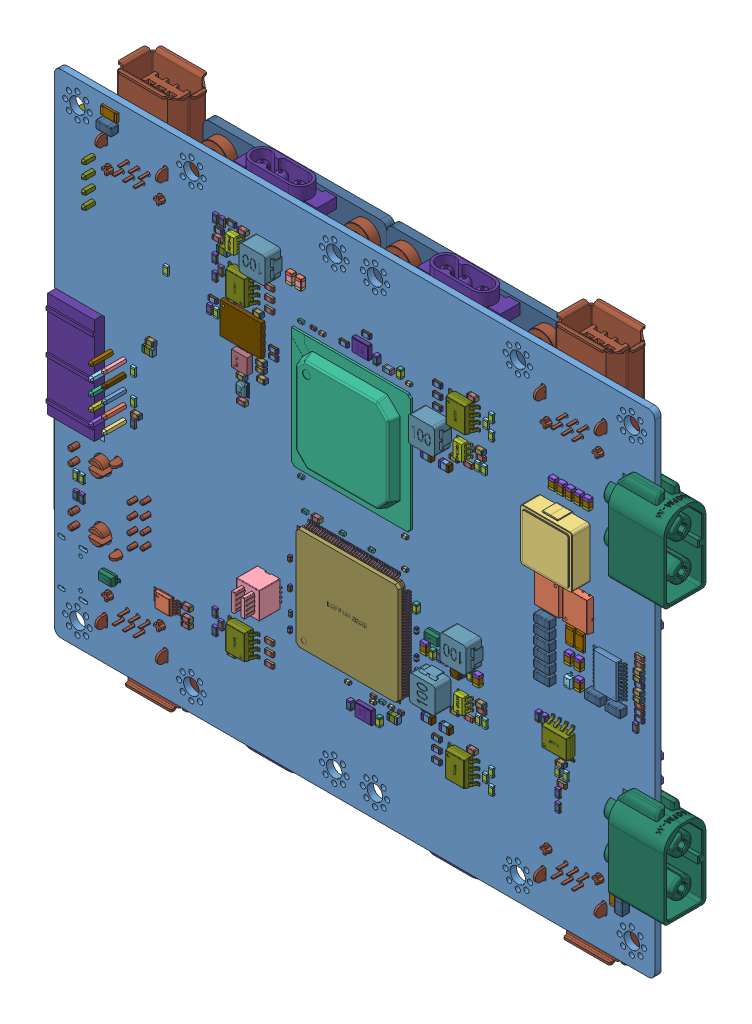
SolidWorks assembly Mother  Board, configuration 默认. Lengths in mm.
Overall size (122.6 102.08 21).
3917 component instances, 207 part files, 0 mates.
Components (placement in the parent):
- Mother  Board.step-1: Mother  Board.step [默认] at origin size (122.6 102.08 21)
  - Board.step-1: Board.step [默认] at origin size (115.82 95 1.22)
    - Open CASCADE STEP translator 6.8 1.1.1.step-1: Open CASCADE STEP translator 6.8 1.1.1.step [默认] at (0 0 -1.2164) size (115.82 95 1.22)
  - C149.step-1: C149.step [默认] at origin size (1.6 0.8 0.8)
    - 5993853984.step-1: 5993853984.step [默认] at (26.0351 21.4629 -1.2164) x (1 0 0) z (0 0 -1) size (1.6 0.8 0.8)
      - Terminal.step-1: Terminal.step [默认] at (-0.8 -0.4 0) size (1.6 0.8 0.8)
        - Open_CASCADE_STEP_translator_6.8_47.1.1.step-1: Open_CASCADE_STEP_translator_6.8_47.1.1.step [默认] at origin size (0.3 0.8 0.8)
        - Open_CASCADE_STEP_translator_6.8_47.1.2.step-1: Open_CASCADE_STEP_translator_6.8_47.1.2.step [默认] at origin size (0.3 0.8 0.8)
      - Mid_Body.step-1: Mid_Body.step [默认] at (-0.8 -0.4 0) size (1 0.8 0.8)
        - Open_CASCADE_STEP_translator_6.8_47.2.1.step-1: Open_CASCADE_STEP_translator_6.8_47.2.1.step [默认] at origin size (1 0.8 0.8)
  - R69.step-1: R69.step [默认] at origin size (1.6 0.8 0.45)
    - 5993853584.step-1: 5993853584.step [默认] at (108.2041 59.0549 -1.2164) x (1 0 0) z (0 0 -1) size (1.6 0.8 0.45)
      - Terminal-1.step-1: Terminal-1.step [默认] at (-0.8 -0.4 0) size (0.3 0.8 0.45)
        - Open_CASCADE_STEP_translator_6.8_21.2.1.step-1: Open_CASCADE_STEP_translator_6.8_21.2.1.step [默认] at origin size (0.3 0.8 0.45)
      - Terminal-1.step-2: Terminal-1.step [默认] at (0.8 0.4 0) x (-1 0 0) z (0 0 1) size (0.3 0.8 0.45)
        - Open_CASCADE_STEP_translator_6.8_21.2.1.step-1: Open_CASCADE_STEP_translator_6.8_21.2.1.step [默认] at origin size (0.3 0.8 0.45)
      - Mid_Body-0.step-1: Mid_Body-0.step [默认] at (-0.8 -0.4 0) size (1.51 0.8 0.36)
      - Mark.step-1: Mark.step [默认] at (-0.5 -0.4 0.405) size (1 0.8 0.05)
  - R68.step-1: R68.step [默认] at origin size (1.6 0.8 0.45)
    - 5993853584.step-1: 5993853584.step [默认] at (108.2041 54.9909 -1.2164) x (1 0 0) z (0 0 -1) size (1.6 0.8 0.45)
      - Terminal-1.step-1: Terminal-1.step [默认] at (-0.8 -0.4 0) size (0.3 0.8 0.45)
        - Open_CASCADE_STEP_translator_6.8_21.2.1.step-1: Open_CASCADE_STEP_translator_6.8_21.2.1.step [默认] at origin size (0.3 0.8 0.45)
      - Terminal-1.step-2: Terminal-1.step [默认] at (0.8 0.4 0) x (-1 0 0) z (0 0 1) size (0.3 0.8 0.45)
        - Open_CASCADE_STEP_translator_6.8_21.2.1.step-1: Open_CASCADE_STEP_translator_6.8_21.2.1.step [默认] at origin size (0.3 0.8 0.45)
      - Mid_Body-0.step-1: Mid_Body-0.step [默认] at (-0.8 -0.4 0) size (1.51 0.8 0.36)
      - Mark.step-1: Mark.step [默认] at (-0.5 -0.4 0.405) size (1 0.8 0.05)
  - R67.step-1: R67.step [默认] at origin size (1.6 0.8 0.45)
    - 5993853584.step-1: 5993853584.step [默认] at (108.2041 33.1469 -1.2164) x (1 0 0) z (0 0 -1) size (1.6 0.8 0.45)
      - Terminal-1.step-1: Terminal-1.step [默认] at (-0.8 -0.4 0) size (0.3 0.8 0.45)
        - Open_CASCADE_STEP_translator_6.8_21.2.1.step-1: Open_CASCADE_STEP_translator_6.8_21.2.1.step [默认] at origin size (0.3 0.8 0.45)
      - Terminal-1.step-2: Terminal-1.step [默认] at (0.8 0.4 0) x (-1 0 0) z (0 0 1) size (0.3 0.8 0.45)
        - Open_CASCADE_STEP_translator_6.8_21.2.1.step-1: Open_CASCADE_STEP_translator_6.8_21.2.1.step [默认] at origin size (0.3 0.8 0.45)
      - Mid_Body-0.step-1: Mid_Body-0.step [默认] at (-0.8 -0.4 0) size (1.51 0.8 0.36)
      - Mark.step-1: Mark.step [默认] at (-0.5 -0.4 0.405) size (1 0.8 0.05)
  - R66.step-1: R66.step [默认] at origin size (1.6 0.8 0.45)
    - 5993853584.step-1: 5993853584.step [默认] at (108.2041 28.9559 -1.2164) x (1 0 0) z (0 0 -1) size (1.6 0.8 0.45)
      - Terminal-1.step-1: Terminal-1.step [默认] at (-0.8 -0.4 0) size (0.3 0.8 0.45)
        - Open_CASCADE_STEP_translator_6.8_21.2.1.step-1: Open_CASCADE_STEP_translator_6.8_21.2.1.step [默认] at origin size (0.3 0.8 0.45)
      - Terminal-1.step-2: Terminal-1.step [默认] at (0.8 0.4 0) x (-1 0 0) z (0 0 1) size (0.3 0.8 0.45)
        - Open_CASCADE_STEP_translator_6.8_21.2.1.step-1: Open_CASCADE_STEP_translator_6.8_21.2.1.step [默认] at origin size (0.3 0.8 0.45)
      - Mid_Body-0.step-1: Mid_Body-0.step [默认] at (-0.8 -0.4 0) size (1.51 0.8 0.36)
      - Mark.step-1: Mark.step [默认] at (-0.5 -0.4 0.405) size (1 0.8 0.05)
  - LED4.step-1: LED4.step [默认] at origin size (1.16 1.62 0.6)
    - User_Library-GSideLED.step-1: User_Library-GSideLED.step [默认] at (109.6341 58.4995 -1.2164) x (0 1 0) z (0 0 -1) size (1.62 1.16 0.6)
  - LED3.step-1: LED3.step [默认] at origin size (1.16 1.62 0.6)
    - User_Library-GSideLED.step-1: User_Library-GSideLED.step [默认] at (109.6341 54.4355 -1.2164) x (0 1 0) z (0 0 -1) size (1.62 1.16 0.6)
  - LED2.step-1: LED2.step [默认] at origin size (1.16 1.62 0.6)
    - User_Library-GSideLED.step-1: User_Library-GSideLED.step [默认] at (109.6341 32.5915 -1.2164) x (0 1 0) z (0 0 -1) size (1.62 1.16 0.6)
  - LED1.step-1: LED1.step [默认] at origin size (1.16 1.62 0.6)
    - User_Library-GSideLED.step-1: User_Library-GSideLED.step [默认] at (109.6341 28.5275 -1.2164) x (0 1 0) z (0 0 -1) size (1.62 1.16 0.6)
  - R65.step-1: R65.step [默认] at origin size (3.1 1.55 0.47)
    - User_Library-R1206.step-1: User_Library-R1206.step [默认] at (6.4771 88.1381 0) x (1 0 0) z (0 0 1) size (3.1 1.55 0.47)
  - C148.step-1: C148.step [默认] at origin size (3 1.5 1.5)
    - (______).step-1: (______).step [默认] at (6.4769 86.2329 0) x (0 -1 0) z (0 0 1) size (1.5 3 1.5)
  - R64.step-1: R64.step [默认] at origin size (1.55 3.1 0.47)
    - User_Library-R1206.step-1: User_Library-R1206.step [默认] at (103.8859 5.9691 0) x (0 1 0) z (0 0 1) size (3.1 1.55 0.47)
  - C116.step-1: C116.step [默认] at origin size (1.5 3 1.5)
    - (______).step-1: (______).step [默认] at (105.7911 5.9689 0) x (1 0 0) z (0 0 1) size (1.5 3 1.5)
  - U10.step-1: U10.step [默认] at origin size (21.4 15.88 16.5)
    - HanRun-HR911105A.step-1: HanRun-HR911105A.step [默认] at (-6.0265 14.8679 -15) x (0 1 0) z (-1 0 0) size (15.88 16.5 21.4)
  - U15.step-1: U15.step [默认] at origin size (22 22 1.45)
    - LQFP144-20x20.step-1: LQFP144-20x20.step [默认] at (53.4654 28.321 0) x (1 0 0) z (0 0 1) size (22 22 1.45)
      - LQFP144_20x20______.step-1: LQFP144_20x20______.step [默认] at origin size (20 20 1.4)
      - _____0.25.step-1: _____0.25.step [默认] at (8.75 -11 0.05) x (-1 0 0) z (0 0 -1) size (0.25 1.2 0.8)
      - _____0.25.step-2: _____0.25.step [默认] at (8.25 -11 0.05) x (-1 0 0) z (0 0 -1) size (0.25 1.2 0.8)
      - _____0.25.step-3: _____0.25.step [默认] at (7.75 -11 0.05) x (-1 0 0) z (0 0 -1) size (0.25 1.2 0.8)
      - _____0.25.step-4: _____0.25.step [默认] at (7.25 -11 0.05) x (-1 0 0) z (0 0 -1) size (0.25 1.2 0.8)
      - _____0.25.step-5: _____0.25.step [默认] at (6.75 -11 0.05) x (-1 0 0) z (0 0 -1) size (0.25 1.2 0.8)
      - _____0.25.step-6: _____0.25.step [默认] at (6.25 -11 0.05) x (-1 0 0) z (0 0 -1) size (0.25 1.2 0.8)
      - _____0.25.step-7: _____0.25.step [默认] at (5.75 -11 0.05) x (-1 0 0) z (0 0 -1) size (0.25 1.2 0.8)
      - _____0.25.step-8: _____0.25.step [默认] at (5.25 -11 0.05) x (-1 0 0) z (0 0 -1) size (0.25 1.2 0.8)
      - _____0.25.step-9: _____0.25.step [默认] at (4.75 -11 0.05) x (-1 0 0) z (0 0 -1) size (0.25 1.2 0.8)
      - _____0.25.step-10: _____0.25.step [默认] at (4.25 -11 0.05) x (-1 0 0) z (0 0 -1) size (0.25 1.2 0.8)
      - _____0.25.step-11: _____0.25.step [默认] at (3.75 -11 0.05) x (-1 0 0) z (0 0 -1) size (0.25 1.2 0.8)
      - _____0.25.step-12: _____0.25.step [默认] at (3.25 -11 0.05) x (-1 0 0) z (0 0 -1) size (0.25 1.2 0.8)
      - _____0.25.step-13: _____0.25.step [默认] at (2.75 -11 0.05) x (-1 0 0) z (0 0 -1) size (0.25 1.2 0.8)
      - _____0.25.step-14: _____0.25.step [默认] at (2.25 -11 0.05) x (-1 0 0) z (0 0 -1) size (0.25 1.2 0.8)
      - _____0.25.step-15: _____0.25.step [默认] at (1.75 -11 0.05) x (-1 0 0) z (0 0 -1) size (0.25 1.2 0.8)
      - _____0.25.step-16: _____0.25.step [默认] at (1.25 -11 0.05) x (-1 0 0) z (0 0 -1) size (0.25 1.2 0.8)
      - _____0.25.step-17: _____0.25.step [默认] at (0.75 -11 0.05) x (-1 0 0) z (0 0 -1) size (0.25 1.2 0.8)
      - _____0.25.step-18: _____0.25.step [默认] at (0.25 -11 0.05) x (-1 0 0) z (0 0 -1) size (0.25 1.2 0.8)
      - _____0.25.step-19: _____0.25.step [默认] at (-0.25 -11 0.05) x (-1 0 0) z (0 0 -1) size (0.25 1.2 0.8)
      - _____0.25.step-20: _____0.25.step [默认] at (-0.75 -11 0.05) x (-1 0 0) z (0 0 -1) size (0.25 1.2 0.8)
      - _____0.25.step-21: _____0.25.step [默认] at (-1.25 -11 0.05) x (-1 0 0) z (0 0 -1) size (0.25 1.2 0.8)
      - _____0.25.step-22: _____0.25.step [默认] at (-1.75 -11 0.05) x (-1 0 0) z (0 0 -1) size (0.25 1.2 0.8)
      - _____0.25.step-23: _____0.25.step [默认] at (-2.25 -11 0.05) x (-1 0 0) z (0 0 -1) size (0.25 1.2 0.8)
      - _____0.25.step-24: _____0.25.step [默认] at (-2.75 -11 0.05) x (-1 0 0) z (0 0 -1) size (0.25 1.2 0.8)
      - _____0.25.step-25: _____0.25.step [默认] at (-3.25 -11 0.05) x (-1 0 0) z (0 0 -1) size (0.25 1.2 0.8)
      - _____0.25.step-26: _____0.25.step [默认] at (-3.75 -11 0.05) x (-1 0 0) z (0 0 -1) size (0.25 1.2 0.8)
      - _____0.25.step-27: _____0.25.step [默认] at (-4.25 -11 0.05) x (-1 0 0) z (0 0 -1) size (0.25 1.2 0.8)
      - _____0.25.step-28: _____0.25.step [默认] at (-4.75 -11 0.05) x (-1 0 0) z (0 0 -1) size (0.25 1.2 0.8)
      - _____0.25.step-29: _____0.25.step [默认] at (-5.25 -11 0.05) x (-1 0 0) z (0 0 -1) size (0.25 1.2 0.8)
      - _____0.25.step-30: _____0.25.step [默认] at (-5.75 -11 0.05) x (-1 0 0) z (0 0 -1) size (0.25 1.2 0.8)
      - _____0.25.step-31: _____0.25.step [默认] at (-6.25 -11 0.05) x (-1 0 0) z (0 0 -1) size (0.25 1.2 0.8)
      - _____0.25.step-32: _____0.25.step [默认] at (-6.75 -11 0.05) x (-1 0 0) z (0 0 -1) size (0.25 1.2 0.8)
      - _____0.25.step-33: _____0.25.step [默认] at (-7.25 -11 0.05) x (-1 0 0) z (0 0 -1) size (0.25 1.2 0.8)
      - _____0.25.step-34: _____0.25.step [默认] at (-7.75 -11 0.05) x (-1 0 0) z (0 0 -1) size (0.25 1.2 0.8)
      - _____0.25.step-35: _____0.25.step [默认] at (-8.25 -11 0.05) x (-1 0 0) z (0 0 -1) size (0.25 1.2 0.8)
      - _____0.25.step-36: _____0.25.step [默认] at (-8.75 -11 0.05) x (-1 0 0) z (0 0 -1) size (0.25 1.2 0.8)
      - _____0.25.step-37: _____0.25.step [默认] at (11 8.75 0.05) x (0 -1 0) z (0 0 -1) size (0.25 1.2 0.8)
      - _____0.25.step-38: _____0.25.step [默认] at (-8.75 11 0.05) x (1 0 0) z (0 0 -1) size (0.25 1.2 0.8)
      - _____0.25.step-39: _____0.25.step [默认] at (-11 -8.75 0.05) x (0 1 0) z (0 0 -1) size (0.25 1.2 0.8)
      - _____0.25.step-40: _____0.25.step [默认] at (11 8.25 0.05) x (0 -1 0) z (0 0 -1) size (0.25 1.2 0.8)
      - _____0.25.step-41: _____0.25.step [默认] at (-8.25 11 0.05) x (1 0 0) z (0 0 -1) size (0.25 1.2 0.8)
      - _____0.25.step-42: _____0.25.step [默认] at (-11 -8.25 0.05) x (0 1 0) z (0 0 -1) size (0.25 1.2 0.8)
      - _____0.25.step-43: _____0.25.step [默认] at (11 7.75 0.05) x (0 -1 0) z (0 0 -1) size (0.25 1.2 0.8)
      - _____0.25.step-44: _____0.25.step [默认] at (-7.75 11 0.05) x (1 0 0) z (0 0 -1) size (0.25 1.2 0.8)
      - _____0.25.step-45: _____0.25.step [默认] at (-11 -7.75 0.05) x (0 1 0) z (0 0 -1) size (0.25 1.2 0.8)
      - _____0.25.step-46: _____0.25.step [默认] at (11 7.25 0.05) x (0 -1 0) z (0 0 -1) size (0.25 1.2 0.8)
      - _____0.25.step-47: _____0.25.step [默认] at (-7.25 11 0.05) x (1 0 0) z (0 0 -1) size (0.25 1.2 0.8)
      - _____0.25.step-48: _____0.25.step [默认] at (-11 -7.25 0.05) x (0 1 0) z (0 0 -1) size (0.25 1.2 0.8)
      - _____0.25.step-49: _____0.25.step [默认] at (11 6.75 0.05) x (0 -1 0) z (0 0 -1) size (0.25 1.2 0.8)
      - _____0.25.step-50: _____0.25.step [默认] at (-6.75 11 0.05) x (1 0 0) z (0 0 -1) size (0.25 1.2 0.8)
      - _____0.25.step-51: _____0.25.step [默认] at (-11 -6.75 0.05) x (0 1 0) z (0 0 -1) size (0.25 1.2 0.8)
      - _____0.25.step-52: _____0.25.step [默认] at (11 6.25 0.05) x (0 -1 0) z (0 0 -1) size (0.25 1.2 0.8)
      - _____0.25.step-53: _____0.25.step [默认] at (-6.25 11 0.05) x (1 0 0) z (0 0 -1) size (0.25 1.2 0.8)
      - _____0.25.step-54: _____0.25.step [默认] at (-11 -6.25 0.05) x (0 1 0) z (0 0 -1) size (0.25 1.2 0.8)
      - _____0.25.step-55: _____0.25.step [默认] at (11 5.75 0.05) x (0 -1 0) z (0 0 -1) size (0.25 1.2 0.8)
      - _____0.25.step-56: _____0.25.step [默认] at (-5.75 11 0.05) x (1 0 0) z (0 0 -1) size (0.25 1.2 0.8)
      - _____0.25.step-57: _____0.25.step [默认] at (-11 -5.75 0.05) x (0 1 0) z (0 0 -1) size (0.25 1.2 0.8)
      - _____0.25.step-58: _____0.25.step [默认] at (11 5.25 0.05) x (0 -1 0) z (0 0 -1) size (0.25 1.2 0.8)
      - _____0.25.step-59: _____0.25.step [默认] at (-5.25 11 0.05) x (1 0 0) z (0 0 -1) size (0.25 1.2 0.8)
      - _____0.25.step-60: _____0.25.step [默认] at (-11 -5.25 0.05) x (0 1 0) z (0 0 -1) size (0.25 1.2 0.8)
      - _____0.25.step-61: _____0.25.step [默认] at (11 4.75 0.05) x (0 -1 0) z (0 0 -1) size (0.25 1.2 0.8)
      - _____0.25.step-62: _____0.25.step [默认] at (-4.75 11 0.05) x (1 0 0) z (0 0 -1) size (0.25 1.2 0.8)
      - _____0.25.step-63: _____0.25.step [默认] at (-11 -4.75 0.05) x (0 1 0) z (0 0 -1) size (0.25 1.2 0.8)
      - _____0.25.step-64: _____0.25.step [默认] at (11 4.25 0.05) x (0 -1 0) z (0 0 -1) size (0.25 1.2 0.8)
      - _____0.25.step-65: _____0.25.step [默认] at (-4.25 11 0.05) x (1 0 0) z (0 0 -1) size (0.25 1.2 0.8)
      - _____0.25.step-66: _____0.25.step [默认] at (-11 -4.25 0.05) x (0 1 0) z (0 0 -1) size (0.25 1.2 0.8)
      - _____0.25.step-67: _____0.25.step [默认] at (11 3.75 0.05) x (0 -1 0) z (0 0 -1) size (0.25 1.2 0.8)
      - _____0.25.step-68: _____0.25.step [默认] at (-3.75 11 0.05) x (1 0 0) z (0 0 -1) size (0.25 1.2 0.8)
      - _____0.25.step-69: _____0.25.step [默认] at (-11 -3.75 0.05) x (0 1 0) z (0 0 -1) size (0.25 1.2 0.8)
      - _____0.25.step-70: _____0.25.step [默认] at (11 3.25 0.05) x (0 -1 0) z (0 0 -1) size (0.25 1.2 0.8)
      - _____0.25.step-71: _____0.25.step [默认] at (-3.25 11 0.05) x (1 0 0) z (0 0 -1) size (0.25 1.2 0.8)
      - _____0.25.step-72: _____0.25.step [默认] at (-11 -3.25 0.05) x (0 1 0) z (0 0 -1) size (0.25 1.2 0.8)
      - _____0.25.step-73: _____0.25.step [默认] at (11 2.75 0.05) x (0 -1 0) z (0 0 -1) size (0.25 1.2 0.8)
      - _____0.25.step-74: _____0.25.step [默认] at (-2.75 11 0.05) x (1 0 0) z (0 0 -1) size (0.25 1.2 0.8)
      - _____0.25.step-75: _____0.25.step [默认] at (-11 -2.75 0.05) x (0 1 0) z (0 0 -1) size (0.25 1.2 0.8)
      - _____0.25.step-76: _____0.25.step [默认] at (11 2.25 0.05) x (0 -1 0) z (0 0 -1) size (0.25 1.2 0.8)
      - _____0.25.step-77: _____0.25.step [默认] at (-2.25 11 0.05) x (1 0 0) z (0 0 -1) size (0.25 1.2 0.8)
      - _____0.25.step-78: _____0.25.step [默认] at (-11 -2.25 0.05) x (0 1 0) z (0 0 -1) size (0.25 1.2 0.8)
      - _____0.25.step-79: _____0.25.step [默认] at (11 1.75 0.05) x (0 -1 0) z (0 0 -1) size (0.25 1.2 0.8)
      - _____0.25.step-80: _____0.25.step [默认] at (-1.75 11 0.05) x (1 0 0) z (0 0 -1) size (0.25 1.2 0.8)
      - _____0.25.step-81: _____0.25.step [默认] at (-11 -1.75 0.05) x (0 1 0) z (0 0 -1) size (0.25 1.2 0.8)
      - _____0.25.step-82: _____0.25.step [默认] at (11 1.25 0.05) x (0 -1 0) z (0 0 -1) size (0.25 1.2 0.8)
      - _____0.25.step-83: _____0.25.step [默认] at (-1.25 11 0.05) x (1 0 0) z (0 0 -1) size (0.25 1.2 0.8)
      - _____0.25.step-84: _____0.25.step [默认] at (-11 -1.25 0.05) x (0 1 0) z (0 0 -1) size (0.25 1.2 0.8)
      - _____0.25.step-85: _____0.25.step [默认] at (11 0.75 0.05) x (0 -1 0) z (0 0 -1) size (0.25 1.2 0.8)
      - _____0.25.step-86: _____0.25.step [默认] at (-0.75 11 0.05) x (1 0 0) z (0 0 -1) size (0.25 1.2 0.8)
      - _____0.25.step-87: _____0.25.step [默认] at (-11 -0.75 0.05) x (0 1 0) z (0 0 -1) size (0.25 1.2 0.8)
      - _____0.25.step-88: _____0.25.step [默认] at (11 0.25 0.05) x (0 -1 0) z (0 0 -1) size (0.25 1.2 0.8)
      - _____0.25.step-89: _____0.25.step [默认] at (-0.25 11 0.05) x (1 0 0) z (0 0 -1) size (0.25 1.2 0.8)
      - _____0.25.step-90: _____0.25.step [默认] at (-11 -0.25 0.05) x (0 1 0) z (0 0 -1) size (0.25 1.2 0.8)
      - _____0.25.step-91: _____0.25.step [默认] at (11 -0.25 0.05) x (0 -1 0) z (0 0 -1) size (0.25 1.2 0.8)
      - _____0.25.step-92: _____0.25.step [默认] at (0.25 11 0.05) x (1 0 0) z (0 0 -1) size (0.25 1.2 0.8)
      - _____0.25.step-93: _____0.25.step [默认] at (-11 0.25 0.05) x (0 1 0) z (0 0 -1) size (0.25 1.2 0.8)
      - _____0.25.step-94: _____0.25.step [默认] at (11 -0.75 0.05) x (0 -1 0) z (0 0 -1) size (0.25 1.2 0.8)
      - _____0.25.step-95: _____0.25.step [默认] at (0.75 11 0.05) x (1 0 0) z (0 0 -1) size (0.25 1.2 0.8)
      - _____0.25.step-96: _____0.25.step [默认] at (-11 0.75 0.05) x (0 1 0) z (0 0 -1) size (0.25 1.2 0.8)
      - _____0.25.step-97: _____0.25.step [默认] at (11 -1.25 0.05) x (0 -1 0) z (0 0 -1) size (0.25 1.2 0.8)
      - _____0.25.step-98: _____0.25.step [默认] at (1.25 11 0.05) x (1 0 0) z (0 0 -1) size (0.25 1.2 0.8)
      - _____0.25.step-99: _____0.25.step [默认] at (-11 1.25 0.05) x (0 1 0) z (0 0 -1) size (0.25 1.2 0.8)
      - _____0.25.step-100: _____0.25.step [默认] at (11 -1.75 0.05) x (0 -1 0) z (0 0 -1) size (0.25 1.2 0.8)
      - _____0.25.step-101: _____0.25.step [默认] at (1.75 11 0.05) x (1 0 0) z (0 0 -1) size (0.25 1.2 0.8)
      - _____0.25.step-102: _____0.25.step [默认] at (-11 1.75 0.05) x (0 1 0) z (0 0 -1) size (0.25 1.2 0.8)
      - _____0.25.step-103: _____0.25.step [默认] at (11 -2.25 0.05) x (0 -1 0) z (0 0 -1) size (0.25 1.2 0.8)
      - _____0.25.step-104: _____0.25.step [默认] at (2.25 11 0.05) x (1 0 0) z (0 0 -1) size (0.25 1.2 0.8)
      - _____0.25.step-105: _____0.25.step [默认] at (-11 2.25 0.05) x (0 1 0) z (0 0 -1) size (0.25 1.2 0.8)
      - _____0.25.step-106: _____0.25.step [默认] at (11 -2.75 0.05) x (0 -1 0) z (0 0 -1) size (0.25 1.2 0.8)
      - _____0.25.step-107: _____0.25.step [默认] at (2.75 11 0.05) x (1 0 0) z (0 0 -1) size (0.25 1.2 0.8)
      - _____0.25.step-108: _____0.25.step [默认] at (-11 2.75 0.05) x (0 1 0) z (0 0 -1) size (0.25 1.2 0.8)
      - _____0.25.step-109: _____0.25.step [默认] at (11 -3.25 0.05) x (0 -1 0) z (0 0 -1) size (0.25 1.2 0.8)
      - _____0.25.step-110: _____0.25.step [默认] at (3.25 11 0.05) x (1 0 0) z (0 0 -1) size (0.25 1.2 0.8)
      - _____0.25.step-111: _____0.25.step [默认] at (-11 3.25 0.05) x (0 1 0) z (0 0 -1) size (0.25 1.2 0.8)
      - _____0.25.step-112: _____0.25.step [默认] at (11 -3.75 0.05) x (0 -1 0) z (0 0 -1) size (0.25 1.2 0.8)
      - _____0.25.step-113: _____0.25.step [默认] at (3.75 11 0.05) x (1 0 0) z (0 0 -1) size (0.25 1.2 0.8)
      - _____0.25.step-114: _____0.25.step [默认] at (-11 3.75 0.05) x (0 1 0) z (0 0 -1) size (0.25 1.2 0.8)
      - _____0.25.step-115: _____0.25.step [默认] at (11 -4.25 0.05) x (0 -1 0) z (0 0 -1) size (0.25 1.2 0.8)
      - _____0.25.step-116: _____0.25.step [默认] at (4.25 11 0.05) x (1 0 0) z (0 0 -1) size (0.25 1.2 0.8)
      - _____0.25.step-117: _____0.25.step [默认] at (-11 4.25 0.05) x (0 1 0) z (0 0 -1) size (0.25 1.2 0.8)
      - _____0.25.step-118: _____0.25.step [默认] at (11 -4.75 0.05) x (0 -1 0) z (0 0 -1) size (0.25 1.2 0.8)
      - _____0.25.step-119: _____0.25.step [默认] at (4.75 11 0.05) x (1 0 0) z (0 0 -1) size (0.25 1.2 0.8)
      - _____0.25.step-120: _____0.25.step [默认] at (-11 4.75 0.05) x (0 1 0) z (0 0 -1) size (0.25 1.2 0.8)
      - _____0.25.step-121: _____0.25.step [默认] at (11 -5.25 0.05) x (0 -1 0) z (0 0 -1) size (0.25 1.2 0.8)
      - _____0.25.step-122: _____0.25.step [默认] at (5.25 11 0.05) x (1 0 0) z (0 0 -1) size (0.25 1.2 0.8)
      - _____0.25.step-123: _____0.25.step [默认] at (-11 5.25 0.05) x (0 1 0) z (0 0 -1) size (0.25 1.2 0.8)
      - _____0.25.step-124: _____0.25.step [默认] at (11 -5.75 0.05) x (0 -1 0) z (0 0 -1) size (0.25 1.2 0.8)
      - _____0.25.step-125: _____0.25.step [默认] at (5.75 11 0.05) x (1 0 0) z (0 0 -1) size (0.25 1.2 0.8)
      - _____0.25.step-126: _____0.25.step [默认] at (-11 5.75 0.05) x (0 1 0) z (0 0 -1) size (0.25 1.2 0.8)
      - _____0.25.step-127: _____0.25.step [默认] at (11 -6.25 0.05) x (0 -1 0) z (0 0 -1) size (0.25 1.2 0.8)
      - _____0.25.step-128: _____0.25.step [默认] at (6.25 11 0.05) x (1 0 0) z (0 0 -1) size (0.25 1.2 0.8)
      - _____0.25.step-129: _____0.25.step [默认] at (-11 6.25 0.05) x (0 1 0) z (0 0 -1) size (0.25 1.2 0.8)
      - _____0.25.step-130: _____0.25.step [默认] at (11 -6.75 0.05) x (0 -1 0) z (0 0 -1) size (0.25 1.2 0.8)
      - _____0.25.step-131: _____0.25.step [默认] at (6.75 11 0.05) x (1 0 0) z (0 0 -1) size (0.25 1.2 0.8)
      - _____0.25.step-132: _____0.25.step [默认] at (-11 6.75 0.05) x (0 1 0) z (0 0 -1) size (0.25 1.2 0.8)
      - _____0.25.step-133: _____0.25.step [默认] at (11 -7.25 0.05) x (0 -1 0) z (0 0 -1) size (0.25 1.2 0.8)
      - _____0.25.step-134: _____0.25.step [默认] at (7.25 11 0.05) x (1 0 0) z (0 0 -1) size (0.25 1.2 0.8)
      - _____0.25.step-135: _____0.25.step [默认] at (-11 7.25 0.05) x (0 1 0) z (0 0 -1) size (0.25 1.2 0.8)
      - _____0.25.step-136: _____0.25.step [默认] at (11 -7.75 0.05) x (0 -1 0) z (0 0 -1) size (0.25 1.2 0.8)
      - _____0.25.step-137: _____0.25.step [默认] at (7.75 11 0.05) x (1 0 0) z (0 0 -1) size (0.25 1.2 0.8)
      - _____0.25.step-138: _____0.25.step [默认] at (-11 7.75 0.05) x (0 1 0) z (0 0 -1) size (0.25 1.2 0.8)
      - _____0.25.step-139: _____0.25.step [默认] at (11 -8.25 0.05) x (0 -1 0) z (0 0 -1) size (0.25 1.2 0.8)
      - _____0.25.step-140: _____0.25.step [默认] at (8.25 11 0.05) x (1 0 0) z (0 0 -1) size (0.25 1.2 0.8)
      - _____0.25.step-141: _____0.25.step [默认] at (-11 8.25 0.05) x (0 1 0) z (0 0 -1) size (0.25 1.2 0.8)
      - _____0.25.step-142: _____0.25.step [默认] at (11 -8.75 0.05) x (0 -1 0) z (0 0 -1) size (0.25 1.2 0.8)
      - _____0.25.step-143: _____0.25.step [默认] at (8.75 11 0.05) x (1 0 0) z (0 0 -1) size (0.25 1.2 0.8)
      - _____0.25.step-144: _____0.25.step [默认] at (-11 8.75 0.05) x (0 1 0) z (0 0 -1) size (0.25 1.2 0.8)
      - LOGO_-0.6.step-1: LOGO_-0.6.step [默认] at (0 -0.0036 0.044) x (-1 0 0) z (0 0 -1) size (1.8 2.12 0.01)
  - JP4.step-1: JP4.step [默认] at origin size (13.7 18.51 8.1)
    - User_Library-XT60PM.step-1: User_Library-XT60PM.step [默认] at (105.8701 16.6369 -0.6) x (0 1 0) z (1 0 0) size (18.51 8.1 13.7)
  - JP3.step-1: JP3.step [默认] at origin size (13.7 18.51 8.1)
    - User_Library-XT60PM.step-1: User_Library-XT60PM.step [默认] at (105.8701 69.4689 -0.6) x (0 1 0) z (1 0 0) size (18.51 8.1 13.7)
  - C82.step-1: C82.step [默认] at origin size (1 0.5 0.5)
    - 5993845664.step-1: 5993845664.step [默认] at (57.9671 51.9279 -1.2164) x (1 0 0) z (0 0 -1) size (1 0.5 0.5)
      - Terminal-2.step-1: Terminal-2.step [默认] at (-0.5 -0.25 0) size (1 0.5 0.5)
        - Open_CASCADE_STEP_translator_6.8_54.1.1.step-1: Open_CASCADE_STEP_translator_6.8_54.1.1.step [默认] at origin size (0.25 0.5 0.5)
        - Open_CASCADE_STEP_translator_6.8_54.1.2.step-1: Open_CASCADE_STEP_translator_6.8_54.1.2.step [默认] at origin size (0.25 0.5 0.5)
      - Mid_Body-1.step-1: Mid_Body-1.step [默认] at (-0.5 -0.25 0) size (0.5 0.5 0.5)
        - Open_CASCADE_STEP_translator_6.8_54.2.1.step-1: Open_CASCADE_STEP_translator_6.8_54.2.1.step [默认] at origin size (0.5 0.5 0.5)
  - C72.step-1: C72.step [默认] at origin size (1 0.5 0.5)
    - 5993845104.step-1: 5993845104.step [默认] at (63.4999 45.9739 0) x (-1 0 0) z (0 0 1) size (1 0.5 0.5)
      - Terminal-3.step-1: Terminal-3.step [默认] at (-0.5 -0.25 0) size (1 0.5 0.5)
        - Open_CASCADE_STEP_translator_6.8_54.1.1-1.step-1: Open_CASCADE_STEP_translator_6.8_54.1.1-1.step [默认] at origin size (0.25 0.5 0.5)
        - Open_CASCADE_STEP_translator_6.8_54.1.2-2.step-1: Open_CASCADE_STEP_translator_6.8_54.1.2-2.step [默认] at origin size (0.25 0.5 0.5)
      - Mid_Body-2.step-1: Mid_Body-2.step [默认] at (-0.5 -0.25 0) size (0.5 0.5 0.5)
        - Open_CASCADE_STEP_translator_6.8_54.2.1-3.step-1: Open_CASCADE_STEP_translator_6.8_54.2.1-3.step [默认] at origin size (0.5 0.5 0.5)
  - C71.step-1: C71.step [默认] at origin size (1 0.5 0.5)
    - 5993847984.step-1: 5993847984.step [默认] at (43.4341 45.9741 0) x (1 0 0) z (0 0 1) size (1 0.5 0.5)
      - Terminal-4.step-1: Terminal-4.step [默认] at (-0.5 -0.25 0) size (1 0.5 0.5)
        - Open_CASCADE_STEP_translator_6.8_54.1.1-4.step-1: Open_CASCADE_STEP_translator_6.8_54.1.1-4.step [默认] at origin size (0.25 0.5 0.5)
        - Open_CASCADE_STEP_translator_6.8_54.1.2-5.step-1: Open_CASCADE_STEP_translator_6.8_54.1.2-5.step [默认] at origin size (0.25 0.5 0.5)
      - Mid_Body-3.step-1: Mid_Body-3.step [默认] at (-0.5 -0.25 0) size (0.5 0.5 0.5)
        - Open_CASCADE_STEP_translator_6.8_54.2.1-6.step-1: Open_CASCADE_STEP_translator_6.8_54.2.1-6.step [默认] at origin size (0.5 0.5 0.5)
  - C70.step-1: C70.step [默认] at origin size (1 0.5 0.5)
    - 5993845104.step-1: 5993845104.step [默认] at (64.2619 71.8819 0) x (-1 0 0) z (0 0 1) size (1 0.5 0.5)
      - Terminal-3.step-1: Terminal-3.step [默认] at (-0.5 -0.25 0) size (1 0.5 0.5)
        - Open_CASCADE_STEP_translator_6.8_54.1.1-1.step-1: Open_CASCADE_STEP_translator_6.8_54.1.1-1.step [默认] at origin size (0.25 0.5 0.5)
        - Open_CASCADE_STEP_translator_6.8_54.1.2-2.step-1: Open_CASCADE_STEP_translator_6.8_54.1.2-2.step [默认] at origin size (0.25 0.5 0.5)
      - Mid_Body-2.step-1: Mid_Body-2.step [默认] at (-0.5 -0.25 0) size (0.5 0.5 0.5)
        - Open_CASCADE_STEP_translator_6.8_54.2.1-3.step-1: Open_CASCADE_STEP_translator_6.8_54.2.1-3.step [默认] at origin size (0.5 0.5 0.5)
  - C64.step-1: C64.step [默认] at origin size (1 0.5 0.5)
    - 5993847984.step-1: 5993847984.step [默认] at (43.4341 71.8821 0) x (1 0 0) z (0 0 1) size (1 0.5 0.5)
      - Terminal-4.step-1: Terminal-4.step [默认] at (-0.5 -0.25 0) size (1 0.5 0.5)
        - Open_CASCADE_STEP_translator_6.8_54.1.1-4.step-1: Open_CASCADE_STEP_translator_6.8_54.1.1-4.step [默认] at origin size (0.25 0.5 0.5)
        - Open_CASCADE_STEP_translator_6.8_54.1.2-5.step-1: Open_CASCADE_STEP_translator_6.8_54.1.2-5.step [默认] at origin size (0.25 0.5 0.5)
      - Mid_Body-3.step-1: Mid_Body-3.step [默认] at (-0.5 -0.25 0) size (0.5 0.5 0.5)
        - Open_CASCADE_STEP_translator_6.8_54.2.1-6.step-1: Open_CASCADE_STEP_translator_6.8_54.2.1-6.step [默认] at origin size (0.5 0.5 0.5)
  - C147.step-1: C147.step [默认] at origin size (0.5 1 0.5)
    - 5993846064.step-1: 5993846064.step [默认] at (47.4589 60.4279 -1.2164) x (0 -1 0) z (0 0 -1) size (1 0.5 0.5)
      - Terminal-5.step-1: Terminal-5.step [默认] at (-0.5 -0.25 0) size (1 0.5 0.5)
        - Open_CASCADE_STEP_translator_6.8_54.1.1-7.step-1: Open_CASCADE_STEP_translator_6.8_54.1.1-7.step [默认] at origin size (0.25 0.5 0.5)
        - Open_CASCADE_STEP_translator_6.8_54.1.2-8.step-1: Open_CASCADE_STEP_translator_6.8_54.1.2-8.step [默认] at origin size (0.25 0.5 0.5)
      - Mid_Body-4.step-1: Mid_Body-4.step [默认] at (-0.5 -0.25 0) size (0.5 0.5 0.5)
        - Open_CASCADE_STEP_translator_6.8_54.2.1-9.step-1: Open_CASCADE_STEP_translator_6.8_54.2.1-9.step [默认] at origin size (0.5 0.5 0.5)
  - C100.step-1: C100.step [默认] at origin size (0.5 1 0.5)
    - 5993846064.step-1: 5993846064.step [默认] at (47.4589 53.4279 -1.2164) x (0 -1 0) z (0 0 -1) size (1 0.5 0.5)
      - Terminal-5.step-1: Terminal-5.step [默认] at (-0.5 -0.25 0) size (1 0.5 0.5)
        - Open_CASCADE_STEP_translator_6.8_54.1.1-7.step-1: Open_CASCADE_STEP_translator_6.8_54.1.1-7.step [默认] at origin size (0.25 0.5 0.5)
        - Open_CASCADE_STEP_translator_6.8_54.1.2-8.step-1: Open_CASCADE_STEP_translator_6.8_54.1.2-8.step [默认] at origin size (0.25 0.5 0.5)
      - Mid_Body-4.step-1: Mid_Body-4.step [默认] at (-0.5 -0.25 0) size (0.5 0.5 0.5)
        - Open_CASCADE_STEP_translator_6.8_54.2.1-9.step-1: Open_CASCADE_STEP_translator_6.8_54.2.1-9.step [默认] at origin size (0.5 0.5 0.5)
  - C90.step-1: C90.step [默认] at origin size (1 0.5 0.5)
    - 5993845664.step-1: 5993845664.step [默认] at (55.9671 64.9359 -1.2164) x (1 0 0) z (0 0 -1) size (1 0.5 0.5)
      - Terminal-2.step-1: Terminal-2.step [默认] at (-0.5 -0.25 0) size (1 0.5 0.5)
        - Open_CASCADE_STEP_translator_6.8_54.1.1.step-1: Open_CASCADE_STEP_translator_6.8_54.1.1.step [默认] at origin size (0.25 0.5 0.5)
        - Open_CASCADE_STEP_translator_6.8_54.1.2.step-1: Open_CASCADE_STEP_translator_6.8_54.1.2.step [默认] at origin size (0.25 0.5 0.5)
      - Mid_Body-1.step-1: Mid_Body-1.step [默认] at (-0.5 -0.25 0) size (0.5 0.5 0.5)
        - Open_CASCADE_STEP_translator_6.8_54.2.1.step-1: Open_CASCADE_STEP_translator_6.8_54.2.1.step [默认] at origin size (0.5 0.5 0.5)
  - C146.step-1: C146.step [默认] at origin size (1.6 0.8 0.8)
    - 5993853264.step-1: 5993853264.step [默认] at (14.6049 54.1019 0) x (-1 0 0) z (0 0 1) size (1.6 0.8 0.8)
      - Terminal-6.step-1: Terminal-6.step [默认] at (-0.8 -0.4 0) size (1.6 0.8 0.8)
        - Open_CASCADE_STEP_translator_6.8_47.1.1-10.step-1: Open_CASCADE_STEP_translator_6.8_47.1.1-10.step [默认] at origin size (0.3 0.8 0.8)
        - Open_CASCADE_STEP_translator_6.8_47.1.2-11.step-1: Open_CASCADE_STEP_translator_6.8_47.1.2-11.step [默认] at origin size (0.3 0.8 0.8)
      - Mid_Body-5.step-1: Mid_Body-5.step [默认] at (-0.8 -0.4 0) size (1 0.8 0.8)
        - Open_CASCADE_STEP_translator_6.8_47.2.1-12.step-1: Open_CASCADE_STEP_translator_6.8_47.2.1-12.step [默认] at origin size (1 0.8 0.8)
  - USB1.step-1: USB1.step [默认] at origin size (7.71 9.58 4.16)
    - 698b116-264-211.step-1: 698b116-264-211.step [默认] at (-10.0486 -7.7822 10.2836) x (0 1 0) z (-1 0 0) size (9.58 4.16 7.71)
      - Open CASCADE STEP translator 6.8 1.28.1.1.step-1: Open CASCADE STEP translator 6.8 1.28.1.1.step [默认] at origin size (8.34 3.56 7.05)
      - Open CASCADE STEP translator 6.8 1.28.1.2.step-1: Open CASCADE STEP translator 6.8 1.28.1.2.step [默认] at origin size (0.26 1.45 0.87)
      - Open CASCADE STEP translator 6.8 1.28.1.3.step-1: Open CASCADE STEP translator 6.8 1.28.1.3.step [默认] at origin size (0.26 1.45 0.87)
      - Open CASCADE STEP translator 6.8 1.28.1.4.step-1: Open CASCADE STEP translator 6.8 1.28.1.4.step [默认] at origin size (0.25 1.45 0.87)
      - Open CASCADE STEP translator 6.8 1.28.1.5.step-1: Open CASCADE STEP translator 6.8 1.28.1.5.step [默认] at origin size (0.25 1.45 0.87)
      - Open CASCADE STEP translator 6.8 1.28.1.6.step-1: Open CASCADE STEP translator 6.8 1.28.1.6.step [默认] at origin size (0.25 2.03 6.58)
      - Open CASCADE STEP translator 6.8 1.28.1.7.step-1: Open CASCADE STEP translator 6.8 1.28.1.7.step [默认] at origin size (0.25 2.03 6.58)
      - Open CASCADE STEP translator 6.8 1.28.1.8.step-1: Open CASCADE STEP translator 6.8 1.28.1.8.step [默认] at origin size (0.25 1.57 6.58)
      - Open CASCADE STEP translator 6.8 1.28.1.9.step-1: Open CASCADE STEP translator 6.8 1.28.1.9.step [默认] at origin size (0.25 1.57 6.58)
      - Open CASCADE STEP translator 6.8 1.28.1.10.step-1: Open CASCADE STEP translator 6.8 1.28.1.10.step [默认] at origin size (0.25 0.24 5.71)
      - Open CASCADE STEP translator 6.8 1.28.1.11.step-1: Open CASCADE STEP translator 6.8 1.28.1.11.step [默认] at origin size (0.25 0.24 5.71)
      - Open CASCADE STEP translator 6.8 1.28.1.12.step-1: Open CASCADE STEP translator 6.8 1.28.1.12.step [默认] at origin size (0.85 1.57 7.13)
      - Open CASCADE STEP translator 6.8 1.28.1.13.step-1: Open CASCADE STEP translator 6.8 1.28.1.13.step [默认] at origin size (0.35 2.03 6.78)
      - Open CASCADE STEP translator 6.8 1.28.1.14.step-1: Open CASCADE STEP translator 6.8 1.28.1.14.step [默认] at origin size (0.35 0.24 5.91)
      - Open CASCADE STEP translator 6.8 1.28.1.15.step-1: Open CASCADE STEP translator 6.8 1.28.1.15.step [默认] at origin size (0.35 2.03 6.78)
      - Open CASCADE STEP translator 6.8 1.28.1.16.step-1: Open CASCADE STEP translator 6.8 1.28.1.16.step [默认] at origin size (0.35 0.24 5.91)
      - Open CASCADE STEP translator 6.8 1.28.1.17.step-1: Open CASCADE STEP translator 6.8 1.28.1.17.step [默认] at origin size (0.85 1.57 7.13)
      - Open CASCADE STEP translator 6.8 1.28.1.18.step-1: Open CASCADE STEP translator 6.8 1.28.1.18.step [默认] at origin size (0.25 0.24 4.21)
      - Open CASCADE STEP translator 6.8 1.28.1.19.step-1: Open CASCADE STEP translator 6.8 1.28.1.19.step [默认] at origin size (0.25 0.24 4.21)
      - Open CASCADE STEP translator 6.8 1.28.1.20.step-1: Open CASCADE STEP translator 6.8 1.28.1.20.step [默认] at origin size (1.11 2.03 7.13)
      - Open CASCADE STEP translator 6.8 1.28.1.21.step-1: Open CASCADE STEP translator 6.8 1.28.1.21.step [默认] at origin size (1.12 2.03 7.13)
      - Open CASCADE STEP translator 6.8 1.28.1.22.step-1: Open CASCADE STEP translator 6.8 1.28.1.22.step [默认] at origin size (9.58 4.16 7.53)
  - Y1.step-1: Y1.step [默认] at origin size (3.2 2.5 0.8)
    - XTAL-3225.step-1: XTAL-3225.step [默认] at (53.6579 74.6941 0) x (0 -1 0) z (-1 0 0) size (2.5 0.8 3.2)
  - X2.step-1: X2.step [默认] at origin size (3.2 2.5 0.8)
    - XTAL-3225.step-1: XTAL-3225.step [默认] at (57.4671 11.5389 0) x (0 1 0) z (1 0 0) size (2.5 0.8 3.2)
  - U14.step-1: U14.step [默认] at origin size (8 6 0.88)
    - User_Library-WSON-8_6x8mm.step-1: User_Library-WSON-8_6x8mm.step [默认] at (28.358 67.1299 0) x (1 0 0) z (0 0 1) size (8 6 0.88)
      - Designator14.step-1: Designator14.step [默认] at origin size (8 6 0.81)
        - 858032368.step-1: 858032368.step [默认] at (3.9 -1.9 0.05) size (7.95 6 0.75)
          - Extruded.step-1: Extruded.step [默认] at origin size (7.95 6 0.75)
        - 858032240.step-1: 858032240.step [默认] at (0.2751 0.0001 0) size (0.45 0.45 0.05)
          - Cylinder.step-1: Cylinder.step [默认] at origin size (0.45 0.45 0.05)
        - 858031856.step-1: 858031856.step [默认] at (0.0875 0 0) size (0.38 0.45 0.25)
          - Extruded_2.step-1: Extruded_2.step [默认] at origin size (0.38 0.45 0.25)
        - 858032240.step-2: 858032240.step [默认] at (0.2751 -1.2699 0) size (0.45 0.45 0.05)
          - Cylinder.step-1: Cylinder.step [默认] at origin size (0.45 0.45 0.05)
        - 858031856.step-2: 858031856.step [默认] at (0.0875 -1.27 0) size (0.38 0.45 0.25)
          - Extruded_2.step-1: Extruded_2.step [默认] at origin size (0.38 0.45 0.25)
        - 858032240.step-3: 858032240.step [默认] at (0.2751 -2.5399 0) size (0.45 0.45 0.05)
          - Cylinder.step-1: Cylinder.step [默认] at origin size (0.45 0.45 0.05)
        - 858031856.step-3: 858031856.step [默认] at (0.0875 -2.54 0) size (0.38 0.45 0.25)
          - Extruded_2.step-1: Extruded_2.step [默认] at origin size (0.38 0.45 0.25)
        - 858032240.step-4: 858032240.step [默认] at (0.2751 -3.8099 0) size (0.45 0.45 0.05)
          - Cylinder.step-1: Cylinder.step [默认] at origin size (0.45 0.45 0.05)
        - 858031856.step-4: 858031856.step [默认] at (0.0875 -3.81 0) size (0.38 0.45 0.25)
          - Extruded_2.step-1: Extruded_2.step [默认] at origin size (0.38 0.45 0.25)
        - 858031856.step-5: 858031856.step [默认] at (7.7125 0 0) size (0.38 0.45 0.25)
          - Extruded_2.step-1: Extruded_2.step [默认] at origin size (0.38 0.45 0.25)
        - 858032240.step-5: 858032240.step [默认] at (7.5251 0.0001 0) size (0.45 0.45 0.05)
          - Cylinder.step-1: Cylinder.step [默认] at origin size (0.45 0.45 0.05)
        - 858031856.step-6: 858031856.step [默认] at (7.7125 -1.27 0) size (0.38 0.45 0.25)
          - Extruded_2.step-1: Extruded_2.step [默认] at origin size (0.38 0.45 0.25)
        - 858032240.step-6: 858032240.step [默认] at (7.5251 -1.2699 0) size (0.45 0.45 0.05)
          - Cylinder.step-1: Cylinder.step [默认] at origin size (0.45 0.45 0.05)
        - 858031856.step-7: 858031856.step [默认] at (7.7125 -2.54 0) size (0.38 0.45 0.25)
          - Extruded_2.step-1: Extruded_2.step [默认] at origin size (0.38 0.45 0.25)
        - 858032240.step-7: 858032240.step [默认] at (7.5251 -2.5399 0) size (0.45 0.45 0.05)
          - Cylinder.step-1: Cylinder.step [默认] at origin size (0.45 0.45 0.05)
        - 858031856.step-8: 858031856.step [默认] at (7.7125 -3.81 0) size (0.38 0.45 0.25)
          - Extruded_2.step-1: Extruded_2.step [默认] at origin size (0.38 0.45 0.25)
        - 858032240.step-8: 858032240.step [默认] at (7.5251 -3.8099 0) size (0.45 0.45 0.05)
          - Cylinder.step-1: Cylinder.step [默认] at origin size (0.45 0.45 0.05)
        - 857275360.step-1: 857275360.step [默认] at (0.6 0.4251 0.7) size (0.45 0.45 0.11)
          - Cylinder_2.step-1: Cylinder_2.step [默认] at origin size (0.45 0.45 0.11)
        - 894460672.step-1: 894460672.step [默认] at (3.9001 -1.8999 0) size (4.75 4.9 0.05)
          - Extruded_3.step-1: Extruded_3.step [默认] at origin size (4.75 4.9 0.05)
      - Board-13.step-1: Board-13.step [默认] at (0 0 -0.0711) size (0.01 0.01 0.07)
  - U13.step-1: U13.step [默认] at origin size (23 23 2.5)
    - User_Library-FBGA484.step-1: User_Library-FBGA484.step [默认] at (53.4671 58.9281 0) x (1 0 0) z (0 0 1) size (23 23 2.5)
  - U5.step-1: U5.step [默认] at origin size (3.01 3 1.55)
    - SOT23-6.step-1: SOT23-6.step [默认] at (74.8028 66.5479 0.1) x (0 -1 0) z (0 0 1) size (3 3.01 1.55)
  - U4.step-1: U4.step [默认] at origin size (3.01 3 1.55)
    - SOT23-6.step-1: SOT23-6.step [默认] at (30.8612 79.1211 0.1) x (0 1 0) z (0 0 1) size (3 3.01 1.55)
  - U3.step-1: U3.step [默认] at origin size (3.01 3 1.55)
    - SOT23-6.step-1: SOT23-6.step [默认] at (74.9297 24.2569 0.1) x (0 -1 0) z (0 0 1) size (3 3.01 1.55)
  - R45.step-1: R45.step [默认] at origin size (1 0.5 0.35)
    - 5993847104.step-1: 5993847104.step [默认] at (45.7201 71.8821 0) x (1 0 0) z (0 0 1) size (1 0.5 0.35)
      - Terminal-7.step-1: Terminal-7.step [默认] at (-0.5 -0.25 0) size (0.25 0.5 0.35)
        - Open_CASCADE_STEP_translator_6.8_20.2.1.step-1: Open_CASCADE_STEP_translator_6.8_20.2.1.step [默认] at origin size (0.25 0.5 0.35)
      - Terminal-7.step-2: Terminal-7.step [默认] at (0.5 0.25 0) x (-1 0 0) z (0 0 1) size (0.25 0.5 0.35)
        - Open_CASCADE_STEP_translator_6.8_20.2.1.step-1: Open_CASCADE_STEP_translator_6.8_20.2.1.step [默认] at origin size (0.25 0.5 0.35)
      - Mid_Body-14.step-1: Mid_Body-14.step [默认] at (-0.5 -0.25 0) size (0.93 0.5 0.28)
      - Mark-15.step-1: Mark-15.step [默认] at (-0.25 -0.25 0.315) size (0.5 0.5 0.03)
  - R62.step-1: R62.step [默认] at origin size (1 0.5 0.35)
    - 5993847504.step-1: 5993847504.step [默认] at (57.2769 16.1289 0) x (-1 0 0) z (0 0 1) size (1 0.5 0.35)
      - Terminal-8.step-1: Terminal-8.step [默认] at (-0.5 -0.25 0) size (0.25 0.5 0.35)
        - Open_CASCADE_STEP_translator_6.8_20.2.1-16.step-1: Open_CASCADE_STEP_translator_6.8_20.2.1-16.step [默认] at origin size (0.25 0.5 0.35)
      - Terminal-8.step-2: Terminal-8.step [默认] at (0.5 0.25 0) x (-1 0 0) z (0 0 1) size (0.25 0.5 0.35)
        - Open_CASCADE_STEP_translator_6.8_20.2.1-16.step-1: Open_CASCADE_STEP_translator_6.8_20.2.1-16.step [默认] at origin size (0.25 0.5 0.35)
      - Mid_Body-17.step-1: Mid_Body-17.step [默认] at (-0.5 -0.25 0) size (0.93 0.5 0.28)
      - Mark-18.step-1: Mark-18.step [默认] at (-0.25 -0.25 0.315) size (0.5 0.5 0.03)
  - R61.step-1: R61.step [默认] at origin size (0.5 1 0.35)
    - 5993847264.step-1: 5993847264.step [默认] at (65.6591 24.5109 0) x (0 -1 0) z (0 0 1) size (1 0.5 0.35)
      - Terminal-9.step-1: Terminal-9.step [默认] at (-0.5 -0.25 0) size (0.25 0.5 0.35)
        - Open_CASCADE_STEP_translator_6.8_20.2.1-19.step-1: Open_CASCADE_STEP_translator_6.8_20.2.1-19.step [默认] at origin size (0.25 0.5 0.35)
      - Terminal-9.step-2: Terminal-9.step [默认] at (0.5 0.25 0) x (-1 0 0) z (0 0 1) size (0.25 0.5 0.35)
        - Open_CASCADE_STEP_translator_6.8_20.2.1-19.step-1: Open_CASCADE_STEP_translator_6.8_20.2.1-19.step [默认] at origin size (0.25 0.5 0.35)
      - Mid_Body-20.step-1: Mid_Body-20.step [默认] at (-0.5 -0.25 0) size (0.93 0.5 0.28)
      - Mark-21.step-1: Mark-21.step [默认] at (-0.25 -0.25 0.315) size (0.5 0.5 0.03)
  - R60.step-1: R60.step [默认] at origin size (0.5 1 0.35)
    - 5993847264.step-1: 5993847264.step [默认] at (41.2751 21.9709 0) x (0 -1 0) z (0 0 1) size (1 0.5 0.35)
      - Terminal-9.step-1: Terminal-9.step [默认] at (-0.5 -0.25 0) size (0.25 0.5 0.35)
        - Open_CASCADE_STEP_translator_6.8_20.2.1-19.step-1: Open_CASCADE_STEP_translator_6.8_20.2.1-19.step [默认] at origin size (0.25 0.5 0.35)
      - Terminal-9.step-2: Terminal-9.step [默认] at (0.5 0.25 0) x (-1 0 0) z (0 0 1) size (0.25 0.5 0.35)
        - Open_CASCADE_STEP_translator_6.8_20.2.1-19.step-1: Open_CASCADE_STEP_translator_6.8_20.2.1-19.step [默认] at origin size (0.25 0.5 0.35)
      - Mid_Body-20.step-1: Mid_Body-20.step [默认] at (-0.5 -0.25 0) size (0.93 0.5 0.28)
      - Mark-21.step-1: Mark-21.step [默认] at (-0.25 -0.25 0.315) size (0.5 0.5 0.03)
  - R59.step-1: R59.step [默认] at origin size (1 0.5 0.35)
    - 5993847104.step-1: 5993847104.step [默认] at (62.6111 16.1291 0) x (1 0 0) z (0 0 1) size (1 0.5 0.35)
      - Terminal-7.step-1: Terminal-7.step [默认] at (-0.5 -0.25 0) size (0.25 0.5 0.35)
        - Open_CASCADE_STEP_translator_6.8_20.2.1.step-1: Open_CASCADE_STEP_translator_6.8_20.2.1.step [默认] at origin size (0.25 0.5 0.35)
      - Terminal-7.step-2: Terminal-7.step [默认] at (0.5 0.25 0) x (-1 0 0) z (0 0 1) size (0.25 0.5 0.35)
        - Open_CASCADE_STEP_translator_6.8_20.2.1.step-1: Open_CASCADE_STEP_translator_6.8_20.2.1.step [默认] at origin size (0.25 0.5 0.35)
      - Mid_Body-14.step-1: Mid_Body-14.step [默认] at (-0.5 -0.25 0) size (0.93 0.5 0.28)
      - Mark-15.step-1: Mark-15.step [默认] at (-0.25 -0.25 0.315) size (0.5 0.5 0.03)
  - R58.step-1: R58.step [默认] at origin size (1.6 0.8 0.45)
    - 5993842144.step-1: 5993842144.step [默认] at (51.6891 72.3901 0) x (1 0 0) z (0 0 1) size (1.6 0.8 0.45)
      - Terminal-10.step-1: Terminal-10.step [默认] at (-0.8 -0.4 0) size (0.3 0.8 0.45)
        - Open_CASCADE_STEP_translator_6.8_21.2.1-22.step-1: Open_CASCADE_STEP_translator_6.8_21.2.1-22.step [默认] at origin size (0.3 0.8 0.45)
      - Terminal-10.step-2: Terminal-10.step [默认] at (0.8 0.4 0) x (-1 0 0) z (0 0 1) size (0.3 0.8 0.45)
        - Open_CASCADE_STEP_translator_6.8_21.2.1-22.step-1: Open_CASCADE_STEP_translator_6.8_21.2.1-22.step [默认] at origin size (0.3 0.8 0.45)
      - Mid_Body-23.step-1: Mid_Body-23.step [默认] at (-0.8 -0.4 0) size (1.51 0.8 0.36)
      - Mark-24.step-1: Mark-24.step [默认] at (-0.5 -0.4 0.405) size (1 0.8 0.05)
  - R57.step-1: R57.step [默认] at origin size (1.6 0.8 0.45)
    - 5993842144.step-1: 5993842144.step [默认] at (56.0071 75.9461 0) x (1 0 0) z (0 0 1) size (1.6 0.8 0.45)
      - Terminal-10.step-1: Terminal-10.step [默认] at (-0.8 -0.4 0) size (0.3 0.8 0.45)
        - Open_CASCADE_STEP_translator_6.8_21.2.1-22.step-1: Open_CASCADE_STEP_translator_6.8_21.2.1-22.step [默认] at origin size (0.3 0.8 0.45)
      - Terminal-10.step-2: Terminal-10.step [默认] at (0.8 0.4 0) x (-1 0 0) z (0 0 1) size (0.3 0.8 0.45)
        - Open_CASCADE_STEP_translator_6.8_21.2.1-22.step-1: Open_CASCADE_STEP_translator_6.8_21.2.1-22.step [默认] at origin size (0.3 0.8 0.45)
      - Mid_Body-23.step-1: Mid_Body-23.step [默认] at (-0.8 -0.4 0) size (1.51 0.8 0.36)
      - Mark-24.step-1: Mark-24.step [默认] at (-0.5 -0.4 0.405) size (1 0.8 0.05)
